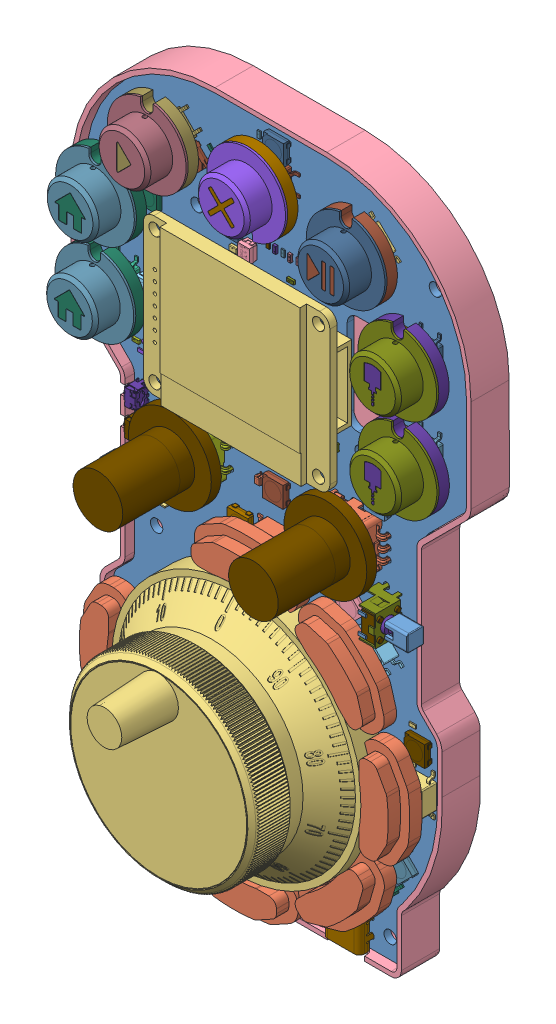
SolidWorks assembly jog3k, configuration Default. Lengths in mm.
Overall size (115.24 180.92 49.48).
240 component instances, 221 part files, 38 mates.
Components (placement in the parent):
- I2C_Jog_Controller-4: I2C_Jog_Controller [Default] at origin size (94.01 162 28.4)
  - Open CASCADE STEP translator 7.5 412-1: Open CASCADE STEP translator 7.5 412 [Default] at origin size (94.01 162 1.63)
  - Open CASCADE STEP translator 7.5 413-1: Open CASCADE STEP translator 7.5 413 [Default] at origin size (10 6 5.08)
  - Open CASCADE STEP translator 7.5 414-1: Open CASCADE STEP translator 7.5 414 [Default] at origin size (6 10 5.08)
  - Open CASCADE STEP translator 7.5 415-1: Open CASCADE STEP translator 7.5 415 [Default] at origin size (6 10 5.08)
  - Open CASCADE STEP translator 7.5 416-1: Open CASCADE STEP translator 7.5 416 [Default] at origin size (10 6 5.08)
  - Open CASCADE STEP translator 7.5 417-1: Open CASCADE STEP translator 7.5 417 [Default] at origin size (1.7 0.8 0.58)
  - Open CASCADE STEP translator 7.5 418-1: Open CASCADE STEP translator 7.5 418 [Default] at origin size (1.77 1.77 0.58)
  - Open CASCADE STEP translator 7.5 419-1: Open CASCADE STEP translator 7.5 419 [Default] at origin size (1.77 1.77 0.58)
  - Open CASCADE STEP translator 7.5 420-1: Open CASCADE STEP translator 7.5 420 [Default] at origin size (5 5.4 1.7)
  - Open CASCADE STEP translator 7.5 421-1: Open CASCADE STEP translator 7.5 421 [Default] at origin size (0.8 1.7 0.58)
  - Open CASCADE STEP translator 7.5 422-1: Open CASCADE STEP translator 7.5 422 [Default] at origin size (0.8 1.6 0.31)
  - Open CASCADE STEP translator 7.5 423-1: Open CASCADE STEP translator 7.5 423 [Default] at origin size (0.8 1.6 0.31)
  - Open CASCADE STEP translator 7.5 424-1: Open CASCADE STEP translator 7.5 424 [Default] at origin size (5 5.4 1.7)
  - Open CASCADE STEP translator 7.5 425-1: Open CASCADE STEP translator 7.5 425 [Default] at origin size (6 10 5.08)
  - Open CASCADE STEP translator 7.5 426-1: Open CASCADE STEP translator 7.5 426 [Default] at origin size (1.7 0.8 0.58)
  - Open CASCADE STEP translator 7.5 427-1: Open CASCADE STEP translator 7.5 427 [Default] at origin size (1.6 0.8 0.31)
  - Open CASCADE STEP translator 7.5 428-1: Open CASCADE STEP translator 7.5 428 [Default] at origin size (1.6 0.8 0.31)
  - Open CASCADE STEP translator 7.5 429-1: Open CASCADE STEP translator 7.5 429 [Default] at origin size (5.4 5 1.7)
  - Open CASCADE STEP translator 7.5 430-1: Open CASCADE STEP translator 7.5 430 [Default] at origin size (0.8 1.7 0.58)
  - Open CASCADE STEP translator 7.5 431-1: Open CASCADE STEP translator 7.5 431 [Default] at origin size (0.8 1.6 0.31)
  - Open CASCADE STEP translator 7.5 432-1: Open CASCADE STEP translator 7.5 432 [Default] at origin size (1.6 0.8 0.31)
  - Open CASCADE STEP translator 7.5 433-1: Open CASCADE STEP translator 7.5 433 [Default] at origin size (7.07 7.07 1.7)
  - Open CASCADE STEP translator 7.5 434-1: Open CASCADE STEP translator 7.5 434 [Default] at origin size (10.75 10.75 5.08)
  - Open CASCADE STEP translator 7.5 435-1: Open CASCADE STEP translator 7.5 435 [Default] at origin size (1.7 0.8 0.58)
  - Open CASCADE STEP translator 7.5 436-1: Open CASCADE STEP translator 7.5 436 [Default] at origin size (1.6 0.8 0.31)
  - Open CASCADE STEP translator 7.5 437-1: Open CASCADE STEP translator 7.5 437 [Default] at origin size (1.69 1.7 0.31)
  - Open CASCADE STEP translator 7.5 438-1: Open CASCADE STEP translator 7.5 438 [Default] at origin size (5 5.4 1.7)
  - Open CASCADE STEP translator 7.5 439-1: Open CASCADE STEP translator 7.5 439 [Default] at origin size (6 10 5.08)
  - Open CASCADE STEP translator 7.5 440-1: Open CASCADE STEP translator 7.5 440 [Default] at origin size (0.8 1.7 0.58)
  - Open CASCADE STEP translator 7.5 441-1: Open CASCADE STEP translator 7.5 441 [Default] at origin size (0.8 1.6 0.31)
  - Open CASCADE STEP translator 7.5 442-1: Open CASCADE STEP translator 7.5 442 [Default] at origin size (1.6 0.8 0.31)
  - Open CASCADE STEP translator 7.5 443-1: Open CASCADE STEP translator 7.5 443 [Default] at origin size (7.07 7.07 1.7)
  - Open CASCADE STEP translator 7.5 444-1: Open CASCADE STEP translator 7.5 444 [Default] at origin size (10.75 10.75 5.08)
  - Open CASCADE STEP translator 7.5 445-1: Open CASCADE STEP translator 7.5 445 [Default] at origin size (0.8 1.7 0.58)
  - Open CASCADE STEP translator 7.5 446-1: Open CASCADE STEP translator 7.5 446 [Default] at origin size (0.8 1.6 0.31)
  - Open CASCADE STEP translator 7.5 447-1: Open CASCADE STEP translator 7.5 447 [Default] at origin size (1.69 1.69 0.31)
  - Open CASCADE STEP translator 7.5 448-1: Open CASCADE STEP translator 7.5 448 [Default] at origin size (5.4 5 1.7)
  - Open CASCADE STEP translator 7.5 449-1: Open CASCADE STEP translator 7.5 449 [Default] at origin size (0.8 1.7 0.58)
  - Open CASCADE STEP translator 7.5 450-1: Open CASCADE STEP translator 7.5 450 [Default] at origin size (0.8 1.6 0.31)
  - Open CASCADE STEP translator 7.5 451-1: Open CASCADE STEP translator 7.5 451 [Default] at origin size (1.6 0.8 0.31)
  - Open CASCADE STEP translator 7.5 452-1: Open CASCADE STEP translator 7.5 452 [Default] at origin size (5 5.4 1.7)
  - Open CASCADE STEP translator 7.5 453-1: Open CASCADE STEP translator 7.5 453 [Default] at origin size (6 10 5.08)
  - Open CASCADE STEP translator 7.5 454-1: Open CASCADE STEP translator 7.5 454 [Default] at origin size (0.8 1.7 0.58)
  - Open CASCADE STEP translator 7.5 455-1: Open CASCADE STEP translator 7.5 455 [Default] at origin size (0.8 1.6 0.31)
  - Open CASCADE STEP translator 7.5 456-1: Open CASCADE STEP translator 7.5 456 [Default] at origin size (1.6 0.8 0.31)
  - Open CASCADE STEP translator 7.5 457-1: Open CASCADE STEP translator 7.5 457 [Default] at origin size (5.4 5 1.7)
  - Open CASCADE STEP translator 7.5 458-1: Open CASCADE STEP translator 7.5 458 [Default] at origin size (10 6 5.08)
  - Open CASCADE STEP translator 7.5 459-1: Open CASCADE STEP translator 7.5 459 [Default] at origin size (0.8 1.7 0.58)
  - Open CASCADE STEP translator 7.5 460-1: Open CASCADE STEP translator 7.5 460 [Default] at origin size (0.8 1.6 0.31)
  - Open CASCADE STEP translator 7.5 461-1: Open CASCADE STEP translator 7.5 461 [Default] at origin size (0.8 1.6 0.31)
  - Open CASCADE STEP translator 7.5 462-1: Open CASCADE STEP translator 7.5 462 [Default] at origin size (5 5.4 1.7)
  - Open CASCADE STEP translator 7.5 463-1: Open CASCADE STEP translator 7.5 463 [Default] at origin size (6 10 5.08)
  - Open CASCADE STEP translator 7.5 464-1: Open CASCADE STEP translator 7.5 464 [Default] at origin size (0.8 1.7 0.58)
  - Open CASCADE STEP translator 7.5 465-1: Open CASCADE STEP translator 7.5 465 [Default] at origin size (0.8 1.6 0.31)
  - Open CASCADE STEP translator 7.5 466-1: Open CASCADE STEP translator 7.5 466 [Default] at origin size (1.6 0.8 0.31)
  - Open CASCADE STEP translator 7.5 467-1: Open CASCADE STEP translator 7.5 467 [Default] at origin size (7.07 7.07 1.7)
  - Open CASCADE STEP translator 7.5 468-1: Open CASCADE STEP translator 7.5 468 [Default] at origin size (10.75 10.75 5.08)
  - Open CASCADE STEP translator 7.5 469-1: Open CASCADE STEP translator 7.5 469 [Default] at origin size (0.8 1.7 0.58)
  - Open CASCADE STEP translator 7.5 470-1: Open CASCADE STEP translator 7.5 470 [Default] at origin size (0.8 1.6 0.31)
  - Open CASCADE STEP translator 7.5 471-1: Open CASCADE STEP translator 7.5 471 [Default] at origin size (1.7 1.69 0.31)
  - Open CASCADE STEP translator 7.5 472-1: Open CASCADE STEP translator 7.5 472 [Default] at origin size (5 5.4 1.7)
  - Open CASCADE STEP translator 7.5 473-1: Open CASCADE STEP translator 7.5 473 [Default] at origin size (0.8 1.7 0.58)
  - Open CASCADE STEP translator 7.5 474-1: Open CASCADE STEP translator 7.5 474 [Default] at origin size (0.8 1.6 0.31)
  - Open CASCADE STEP translator 7.5 475-1: Open CASCADE STEP translator 7.5 475 [Default] at origin size (1.6 0.8 0.31)
  - Open CASCADE STEP translator 7.5 476-1: Open CASCADE STEP translator 7.5 476 [Default] at origin size (7.07 7.07 1.7)
  - Open CASCADE STEP translator 7.5 477-1: Open CASCADE STEP translator 7.5 477 [Default] at origin size (10.75 10.75 5.08)
  - Open CASCADE STEP translator 7.5 478-1: Open CASCADE STEP translator 7.5 478 [Default] at origin size (0.8 1.7 0.58)
  - Open CASCADE STEP translator 7.5 479-1: Open CASCADE STEP translator 7.5 479 [Default] at origin size (0.8 1.6 0.31)
  - Open CASCADE STEP translator 7.5 480-1: Open CASCADE STEP translator 7.5 480 [Default] at origin size (1.7 1.69 0.31)
  - Open CASCADE STEP translator 7.5 481-1: Open CASCADE STEP translator 7.5 481 [Default] at origin size (6.25 8.7 11.7)
  - Open CASCADE STEP translator 7.5 482-1: Open CASCADE STEP translator 7.5 482 [Default] at origin size (4 3.5 3.5)
  - Open CASCADE STEP translator 7.5 483-1: Open CASCADE STEP translator 7.5 483 [Default] at origin size (3.91 6.01 6.01)
  - Open CASCADE STEP translator 7.5 484-1: Open CASCADE STEP translator 7.5 484 [Default] at origin size (1.9 5.2 11.6)
  - Open CASCADE STEP translator 7.5 485-1: Open CASCADE STEP translator 7.5 485 [Default] at origin size (3 0.02 4.74)
  - Open CASCADE STEP translator 7.5 486-1: Open CASCADE STEP translator 7.5 486 [Default] at origin size (6.25 8.7 11.7)
  - Open CASCADE STEP translator 7.5 487-1: Open CASCADE STEP translator 7.5 487 [Default] at origin size (4 3.5 3.5)
  - Open CASCADE STEP translator 7.5 488-1: Open CASCADE STEP translator 7.5 488 [Default] at origin size (3.91 6.01 6.01)
  - Open CASCADE STEP translator 7.5 489-1: Open CASCADE STEP translator 7.5 489 [Default] at origin size (1.9 5.2 11.6)
  - Open CASCADE STEP translator 7.5 490-1: Open CASCADE STEP translator 7.5 490 [Default] at origin size (3 0.02 4.74)
  - Open CASCADE STEP translator 7.5 491-1: Open CASCADE STEP translator 7.5 491 [Default] at origin size (7.31 7.31 2.01)
  - Open CASCADE STEP translator 7.5 492-1: Open CASCADE STEP translator 7.5 492 [Default] at origin size (1.77 1.77 0.58)
  - Open CASCADE STEP translator 7.5 493-1: Open CASCADE STEP translator 7.5 493 [Default] at origin size (1.77 1.77 0.58)
  - Open CASCADE STEP translator 7.5 494-1: Open CASCADE STEP translator 7.5 494 [Default] at origin size (1.69 1.69 0.31)
  - Open CASCADE STEP translator 7.5 495-1: Open CASCADE STEP translator 7.5 495 [Default] at origin size (1.69 1.7 0.31)
  - Open CASCADE STEP translator 7.5 496-1: Open CASCADE STEP translator 7.5 496 [Default] at origin size (1.7 1.69 0.31)
  - Open CASCADE STEP translator 7.5 497-1: Open CASCADE STEP translator 7.5 497 [Default] at origin size (1.7 0.8 0.58)
  - Open CASCADE STEP translator 7.5 498-1: Open CASCADE STEP translator 7.5 498 [Default] at origin size (1.6 0.8 0.31)
  - Open CASCADE STEP translator 7.5 499-1: Open CASCADE STEP translator 7.5 499 [Default] at origin size (1.7 0.8 0.58)
  - Open CASCADE STEP translator 7.5 500-1: Open CASCADE STEP translator 7.5 500 [Default] at origin size (0.8 1.7 0.58)
  - Open CASCADE STEP translator 7.5 501-1: Open CASCADE STEP translator 7.5 501 [Default] at origin size (0.8 1.7 0.58)
  - Open CASCADE STEP translator 7.5 502-1: Open CASCADE STEP translator 7.5 502 [Default] at origin size (1.7 0.8 0.58)
  - Open CASCADE STEP translator 7.5 503-1: Open CASCADE STEP translator 7.5 503 [Default] at origin size (1.7 0.8 0.58)
  - Open CASCADE STEP translator 7.5 504-1: Open CASCADE STEP translator 7.5 504 [Default] at origin size (1.7 0.8 0.58)
  - Open CASCADE STEP translator 7.5 505-1: Open CASCADE STEP translator 7.5 505 [Default] at origin size (0.8 1.6 0.31)
  - Open CASCADE STEP translator 7.5 506-1: Open CASCADE STEP translator 7.5 506 [Default] at origin size (1.6 0.8 0.31)
  - Open CASCADE STEP translator 7.5 507-1: Open CASCADE STEP translator 7.5 507 [Default] at origin size (1.6 0.8 0.31)
  - Open CASCADE STEP translator 7.5 508-1: Open CASCADE STEP translator 7.5 508 [Default] at origin size (1.6 0.8 0.31)
  - Open CASCADE STEP translator 7.5 509-1: Open CASCADE STEP translator 7.5 509 [Default] at origin size (1.6 0.8 0.31)
  - Open CASCADE STEP translator 7.5 510-1: Open CASCADE STEP translator 7.5 510 [Default] at origin size (1.6 0.8 0.31)
  - Open CASCADE STEP translator 7.5 511-1: Open CASCADE STEP translator 7.5 511 [Default] at origin size (3.1 1.8 1.25)
  - Open CASCADE STEP translator 7.5 512-1: Open CASCADE STEP translator 7.5 512 [Default] at origin size (5.4 5 1.7)
  - Open CASCADE STEP translator 7.5 513-1: Open CASCADE STEP translator 7.5 513 [Default] at origin size (0.8 1.7 0.58)
  - Open CASCADE STEP translator 7.5 514-1: Open CASCADE STEP translator 7.5 514 [Default] at origin size (0.8 1.7 0.58)
  - Open CASCADE STEP translator 7.5 515-1: Open CASCADE STEP translator 7.5 515 [Default] at origin size (1.77 1.77 0.58)
  - Open CASCADE STEP translator 7.5 516-1: Open CASCADE STEP translator 7.5 516 [Default] at origin size (1.77 1.77 0.58)
  - Open CASCADE STEP translator 7.5 517-1: Open CASCADE STEP translator 7.5 517 [Default] at origin size (1.7 0.8 0.58)
  - Open CASCADE STEP translator 7.5 518-1: Open CASCADE STEP translator 7.5 518 [Default] at origin size (1.77 1.77 0.58)
  - Open CASCADE STEP translator 7.5 519-1: Open CASCADE STEP translator 7.5 519 [Default] at origin size (1.77 1.77 0.58)
  - Open CASCADE STEP translator 7.5 520-1: Open CASCADE STEP translator 7.5 520 [Default] at origin size (1.77 1.77 0.58)
  - Open CASCADE STEP translator 7.5 521-1: Open CASCADE STEP translator 7.5 521 [Default] at origin size (1.25 2.74 1.12)
  - Open CASCADE STEP translator 7.5 522-1: Open CASCADE STEP translator 7.5 522 [Default] at origin size (2 1.25 0.8)
  - Open CASCADE STEP translator 7.5 523-1: Open CASCADE STEP translator 7.5 523 [Default] at origin size (2.93 3.7 2.03)
  - Open CASCADE STEP translator 7.5 524-1: Open CASCADE STEP translator 7.5 524 [Default] at origin size (1.25 2 0.8)
  - Open CASCADE STEP translator 7.5 525-1: Open CASCADE STEP translator 7.5 525 [Default] at origin size (1.69 1.7 0.31)
  - Open CASCADE STEP translator 7.5 526-1: Open CASCADE STEP translator 7.5 526 [Default] at origin size (1.69 1.69 0.31)
  - Open CASCADE STEP translator 7.5 527-1: Open CASCADE STEP translator 7.5 527 [Default] at origin size (1.7 1.69 0.31)
  - Open CASCADE STEP translator 7.5 528-1: Open CASCADE STEP translator 7.5 528 [Default] at origin size (1.7 1.69 0.31)
  - Open CASCADE STEP translator 7.5 529-1: Open CASCADE STEP translator 7.5 529 [Default] at origin size (1.69 1.69 0.31)
  - Open CASCADE STEP translator 7.5 530-1: Open CASCADE STEP translator 7.5 530 [Default] at origin size (1.7 1.7 0.31)
  - Open CASCADE STEP translator 7.5 531-1: Open CASCADE STEP translator 7.5 531 [Default] at origin size (1.7 1.69 0.31)
  - Open CASCADE STEP translator 7.5 532-1: Open CASCADE STEP translator 7.5 532 [Default] at origin size (1.7 1.69 0.31)
  - Open CASCADE STEP translator 7.5 533-1: Open CASCADE STEP translator 7.5 533 [Default] at origin size (1.7 1.69 0.31)
  - Open CASCADE STEP translator 7.5 534-1: Open CASCADE STEP translator 7.5 534 [Default] at origin size (1.69 1.69 0.31)
  - Open CASCADE STEP translator 7.5 535-1: Open CASCADE STEP translator 7.5 535 [Default] at origin size (1.7 1.7 0.31)
  - Open CASCADE STEP translator 7.5 536-1: Open CASCADE STEP translator 7.5 536 [Default] at origin size (0.8 1.6 0.31)
  - Open CASCADE STEP translator 7.5 537-1: Open CASCADE STEP translator 7.5 537 [Default] at origin size (0.8 1.6 0.31)
  - Open CASCADE STEP translator 7.5 538-1: Open CASCADE STEP translator 7.5 538 [Default] at origin size (2.3 2.24 0.84)
  - Open CASCADE STEP translator 7.5 539-1: Open CASCADE STEP translator 7.5 539 [Default] at origin size (0.8 1.6 0.31)
  - Open CASCADE STEP translator 7.5 540-1: Open CASCADE STEP translator 7.5 540 [Default] at origin size (0.6 1 0.21)
  - Open CASCADE STEP translator 7.5 541-1: Open CASCADE STEP translator 7.5 541 [Default] at origin size (0.8 1.6 0.31)
  - Open CASCADE STEP translator 7.5 542-1: Open CASCADE STEP translator 7.5 542 [Default] at origin size (1.77 1.77 0.58)
  - Open CASCADE STEP translator 7.5 543-1: Open CASCADE STEP translator 7.5 543 [Default] at origin size (0.8 1.6 0.31)
  - Open CASCADE STEP translator 7.5 544-1: Open CASCADE STEP translator 7.5 544 [Default] at origin size (1.7 0.8 0.58)
  - Open CASCADE STEP translator 7.5 545-1: Open CASCADE STEP translator 7.5 545 [Default] at origin size (1.6 0.8 0.31)
  - Open CASCADE STEP translator 7.5 546-1: Open CASCADE STEP translator 7.5 546 [Default] at origin size (8.94 7.91 4.3)
  - Open CASCADE STEP translator 7.5 547-1: Open CASCADE STEP translator 7.5 547 [Default] at origin size (3.2 2.5 0.8)
  - Open CASCADE STEP translator 7.5 548-1: Open CASCADE STEP translator 7.5 548 [Default] at origin size (3.36 2.66 0.1)
  - Open CASCADE STEP translator 7.5 549-1: Open CASCADE STEP translator 7.5 549 [Default] at origin size (0.88 0.88 0)
  - Open CASCADE STEP translator 7.5 550-1: Open CASCADE STEP translator 7.5 550 [Default] at origin size (9.9 9.9 0.9)
  - Open CASCADE STEP translator 7.5 551-1: Open CASCADE STEP translator 7.5 551 [Default] at origin size (4.28 4.53 0)
  - Open CASCADE STEP translator 7.5 552-1: Open CASCADE STEP translator 7.5 552 [Default] at origin size (0.42 0.42 0.2)
  - Open CASCADE STEP translator 7.5 553-1: Open CASCADE STEP translator 7.5 553 [Default] at origin size (0.42 0.42 0.2)
  - Open CASCADE STEP translator 7.5 554-1: Open CASCADE STEP translator 7.5 554 [Default] at origin size (0.42 0.42 0.2)
  - Open CASCADE STEP translator 7.5 555-1: Open CASCADE STEP translator 7.5 555 [Default] at origin size (0.42 0.42 0.2)
  - Open CASCADE STEP translator 7.5 556-1: Open CASCADE STEP translator 7.5 556 [Default] at origin size (0.42 0.42 0.2)
  - Open CASCADE STEP translator 7.5 557-1: Open CASCADE STEP translator 7.5 557 [Default] at origin size (0.42 0.42 0.2)
  - Open CASCADE STEP translator 7.5 558-1: Open CASCADE STEP translator 7.5 558 [Default] at origin size (0.42 0.42 0.2)
  - Open CASCADE STEP translator 7.5 559-1: Open CASCADE STEP translator 7.5 559 [Default] at origin size (0.42 0.42 0.2)
  - Open CASCADE STEP translator 7.5 560-1: Open CASCADE STEP translator 7.5 560 [Default] at origin size (0.42 0.42 0.2)
  - Open CASCADE STEP translator 7.5 561-1: Open CASCADE STEP translator 7.5 561 [Default] at origin size (0.42 0.42 0.2)
  - Open CASCADE STEP translator 7.5 562-1: Open CASCADE STEP translator 7.5 562 [Default] at origin size (0.42 0.42 0.2)
  - Open CASCADE STEP translator 7.5 563-1: Open CASCADE STEP translator 7.5 563 [Default] at origin size (0.42 0.42 0.2)
  - Open CASCADE STEP translator 7.5 564-1: Open CASCADE STEP translator 7.5 564 [Default] at origin size (0.42 0.42 0.2)
  - Open CASCADE STEP translator 7.5 565-1: Open CASCADE STEP translator 7.5 565 [Default] at origin size (0.42 0.42 0.2)
  - Open CASCADE STEP translator 7.5 566-1: Open CASCADE STEP translator 7.5 566 [Default] at origin size (0.42 0.42 0.2)
  - Open CASCADE STEP translator 7.5 567-1: Open CASCADE STEP translator 7.5 567 [Default] at origin size (0.42 0.42 0.2)
  - Open CASCADE STEP translator 7.5 568-1: Open CASCADE STEP translator 7.5 568 [Default] at origin size (0.42 0.42 0.2)
  - Open CASCADE STEP translator 7.5 569-1: Open CASCADE STEP translator 7.5 569 [Default] at origin size (0.42 0.42 0.2)
  - Open CASCADE STEP translator 7.5 570-1: Open CASCADE STEP translator 7.5 570 [Default] at origin size (0.42 0.42 0.2)
  - Open CASCADE STEP translator 7.5 571-1: Open CASCADE STEP translator 7.5 571 [Default] at origin size (0.42 0.42 0.2)
  - Open CASCADE STEP translator 7.5 572-1: Open CASCADE STEP translator 7.5 572 [Default] at origin size (0.42 0.42 0.2)
  - Open CASCADE STEP translator 7.5 573-1: Open CASCADE STEP translator 7.5 573 [Default] at origin size (0.42 0.42 0.2)
  - Open CASCADE STEP translator 7.5 574-1: Open CASCADE STEP translator 7.5 574 [Default] at origin size (0.42 0.42 0.2)
  - Open CASCADE STEP translator 7.5 575-1: Open CASCADE STEP translator 7.5 575 [Default] at origin size (0.42 0.42 0.2)
  - Open CASCADE STEP translator 7.5 576-1: Open CASCADE STEP translator 7.5 576 [Default] at origin size (0.42 0.42 0.2)
  - Open CASCADE STEP translator 7.5 577-1: Open CASCADE STEP translator 7.5 577 [Default] at origin size (0.42 0.42 0.2)
  - Open CASCADE STEP translator 7.5 578-1: Open CASCADE STEP translator 7.5 578 [Default] at origin size (0.42 0.42 0.2)
  - Open CASCADE STEP translator 7.5 579-1: Open CASCADE STEP translator 7.5 579 [Default] at origin size (0.42 0.42 0.2)
  - Open CASCADE STEP translator 7.5 580-1: Open CASCADE STEP translator 7.5 580 [Default] at origin size (0.42 0.42 0.2)
  - Open CASCADE STEP translator 7.5 581-1: Open CASCADE STEP translator 7.5 581 [Default] at origin size (0.42 0.42 0.2)
  - Open CASCADE STEP translator 7.5 582-1: Open CASCADE STEP translator 7.5 582 [Default] at origin size (0.42 0.42 0.2)
  - Open CASCADE STEP translator 7.5 583-1: Open CASCADE STEP translator 7.5 583 [Default] at origin size (0.42 0.42 0.2)
  - Open CASCADE STEP translator 7.5 584-1: Open CASCADE STEP translator 7.5 584 [Default] at origin size (0.42 0.42 0.2)
  - Open CASCADE STEP translator 7.5 585-1: Open CASCADE STEP translator 7.5 585 [Default] at origin size (0.42 0.42 0.2)
  - Open CASCADE STEP translator 7.5 586-1: Open CASCADE STEP translator 7.5 586 [Default] at origin size (0.42 0.42 0.2)
  - Open CASCADE STEP translator 7.5 587-1: Open CASCADE STEP translator 7.5 587 [Default] at origin size (0.42 0.42 0.2)
  - Open CASCADE STEP translator 7.5 588-1: Open CASCADE STEP translator 7.5 588 [Default] at origin size (0.42 0.42 0.2)
  - Open CASCADE STEP translator 7.5 589-1: Open CASCADE STEP translator 7.5 589 [Default] at origin size (0.42 0.42 0.2)
  - Open CASCADE STEP translator 7.5 590-1: Open CASCADE STEP translator 7.5 590 [Default] at origin size (0.42 0.42 0.2)
  - Open CASCADE STEP translator 7.5 591-1: Open CASCADE STEP translator 7.5 591 [Default] at origin size (0.42 0.42 0.2)
  - Open CASCADE STEP translator 7.5 592-1: Open CASCADE STEP translator 7.5 592 [Default] at origin size (0.42 0.42 0.2)
  - Open CASCADE STEP translator 7.5 593-1: Open CASCADE STEP translator 7.5 593 [Default] at origin size (0.42 0.42 0.2)
  - Open CASCADE STEP translator 7.5 594-1: Open CASCADE STEP translator 7.5 594 [Default] at origin size (0.42 0.42 0.2)
  - Open CASCADE STEP translator 7.5 595-1: Open CASCADE STEP translator 7.5 595 [Default] at origin size (0.42 0.42 0.2)
  - Open CASCADE STEP translator 7.5 596-1: Open CASCADE STEP translator 7.5 596 [Default] at origin size (0.42 0.42 0.2)
  - Open CASCADE STEP translator 7.5 597-1: Open CASCADE STEP translator 7.5 597 [Default] at origin size (0.42 0.42 0.2)
  - Open CASCADE STEP translator 7.5 598-1: Open CASCADE STEP translator 7.5 598 [Default] at origin size (0.42 0.42 0.2)
  - Open CASCADE STEP translator 7.5 599-1: Open CASCADE STEP translator 7.5 599 [Default] at origin size (0.42 0.42 0.2)
  - Open CASCADE STEP translator 7.5 600-1: Open CASCADE STEP translator 7.5 600 [Default] at origin size (0.42 0.42 0.2)
  - Open CASCADE STEP translator 7.5 601-1: Open CASCADE STEP translator 7.5 601 [Default] at origin size (0.42 0.42 0.2)
  - Open CASCADE STEP translator 7.5 602-1: Open CASCADE STEP translator 7.5 602 [Default] at origin size (0.42 0.42 0.2)
  - Open CASCADE STEP translator 7.5 603-1: Open CASCADE STEP translator 7.5 603 [Default] at origin size (0.42 0.42 0.2)
  - Open CASCADE STEP translator 7.5 604-1: Open CASCADE STEP translator 7.5 604 [Default] at origin size (0.42 0.42 0.2)
  - Open CASCADE STEP translator 7.5 605-1: Open CASCADE STEP translator 7.5 605 [Default] at origin size (0.42 0.42 0.2)
  - Open CASCADE STEP translator 7.5 606-1: Open CASCADE STEP translator 7.5 606 [Default] at origin size (0.42 0.42 0.2)
  - Open CASCADE STEP translator 7.5 607-1: Open CASCADE STEP translator 7.5 607 [Default] at origin size (0.42 0.42 0.2)
  - Open CASCADE STEP translator 7.5 608-1: Open CASCADE STEP translator 7.5 608 [Default] at origin size (3.55 4.5 3.8)
  - Open CASCADE STEP translator 7.5 609-1: Open CASCADE STEP translator 7.5 609 [Default] at origin size (3.55 4.5 3.8)
  - Open CASCADE STEP translator 7.5 610-1: Open CASCADE STEP translator 7.5 610 [Default] at origin size (5.4 5 1.7)
  - Open CASCADE STEP translator 7.5 611-1: Open CASCADE STEP translator 7.5 611 [Default] at origin size (14.98 13.1 28.2)
  - Open CASCADE STEP translator 7.5 612-1: Open CASCADE STEP translator 7.5 612 [Default] at origin size (45 37.5 9.4)
  - Open CASCADE STEP translator 7.5 613-1: Open CASCADE STEP translator 7.5 613 [Default] at origin size (5.23 5.23 1.8)
  - Open CASCADE STEP translator 7.5 614-1: Open CASCADE STEP translator 7.5 614 [Default] at origin size (7.8 4.23 1.11)
  - Open CASCADE STEP translator 7.5 616-1: Open CASCADE STEP translator 7.5 616 [Default] at origin size (5.4 5 1.7)
  - Open CASCADE STEP translator 7.5 617-1: Open CASCADE STEP translator 7.5 617 [Default] at origin size (14.98 13.1 28.2)
- halt_button-1: halt_button [Default] at (7.9129 120.3247 -3.7629) x (-1 0 0) z (0 0 1) size (19 18.88 9)
  - Halt Button Cover-1: Halt Button Cover [Default] at (7.9127 9.3246 8.8429) size (19 18.88 6.5)
  - Halt Button Lightpipe-1: Halt Button Lightpipe [Default] at (7.9127 9.3246 8.8429) size (19 18.88 9)
- Hold_button-1: Hold_button [Default] at (18.335 99.1832 -4.6146) size (19 18.88 9)
  - Hold Button Cover-2: Hold Button Cover [Default] at (5.6648 9.8169 9.6946) size (19 18.88 6.5)
  - Hold Button Lightpipe-1: Hold Button Lightpipe [Default] at (5.6648 9.8169 9.6946) size (19 18.88 9)
- start_button-1: start_button [Default] at (-32.4958 98.8123 -8.5785) size (19 18.88 9)
  - Start Button Lightpipe-1: Start Button Lightpipe [Default] at (8.4957 10.1876 13.6585) size (19 18.88 9)
  - Start Button Cover-1: Start Button Cover [Default] at (8.4957 10.1876 13.6585) size (19 18.88 6.5)
- Home_button-1: Home_button [Default] at (-43.1593 60.9431 -3.5645) size (19 18.88 9)
  - Home Button Cover-1: Home Button Cover [Default] at (6.5093 10.7068 8.6445) size (19 18.88 6.5)
  - Home Button Lightpipe-1: Home Button Lightpipe [Default] at (6.5093 10.7068 8.6445) size (19 18.88 9)
- spindle_button-1: spindle_button [Default] at (35.5679 62.8775 -7.999) size (19 18.88 9)
  - Spindle Button Cover-1: Spindle Button Cover [Default] at (0.982 8.4726 13.079) size (19 18.88 6.5)
  - Spindle Button Lightpipe-1: Spindle Button Lightpipe [Default] at (0.982 8.4726 13.079) size (19 18.88 9)
- spindle_button-2: spindle_button [Default] at (35.5179 83.5275 -7.999) size (19 18.88 9)
  - Spindle Button Cover-1: Spindle Button Cover [Default] at (0.982 8.4726 13.079) size (19 18.88 6.5)
  - Spindle Button Lightpipe-1: Spindle Button Lightpipe [Default] at (0.982 8.4726 13.079) size (19 18.88 9)
- Home_button-2: Home_button [Default] at (-43.0093 81.2931 -3.5645) size (19 18.88 9)
  - Home Button Cover-1: Home Button Cover [Default] at (6.5093 10.7068 8.6445) size (19 18.88 6.5)
  - Home Button Lightpipe-1: Home Button Lightpipe [Default] at (6.5093 10.7068 8.6445) size (19 18.88 9)
- simple_rotary_knob^jog3k-1: simple_rotary_knob^jog3k [Default] at (0 0 4.3036) x (1 0 0) z (0 0 1) size (20 20 19.8)
- b32-1010-1: b32-1010 [Default] at (31.675 34.35 4.35) x (0 -1 0) z (0 0 1) size (4 5.5 4)
- b32-1010-2: b32-1010 [Default] at (-31.675 34.35 4.35) x (0 -1 0) z (0 0 -1) size (4 5.5 4)
- simple_rotary_knob^jog3k-2: simple_rotary_knob^jog3k [Default] at (0 92 4.3036) x (-1 0 0) z (0 0 1) size (20 20 19.8)
- simple_direction_button^jog3k-1: simple_direction_button^jog3k [Default] at (0 0 5.08) size (25 57.62 6)
- simple_direction_button^jog3k-2: simple_direction_button^jog3k [Default] at (0 0.0057 5.08) x (0 1 0) z (0 0 1) size (25 57.62 6)
- simple_direction_button^jog3k-3: simple_direction_button^jog3k [Default] at (-0.0005 -0.1857 5.08) x (0 -1 0) z (0 0 1) size (25 57.62 6)
- simple_direction_button^jog3k-4: simple_direction_button^jog3k [Default] at (-0.0084 0 5.08) x (-1 0 0) z (0 0 1) size (25 57.62 6)
- simple_direction_button^jog3k-5: simple_direction_button^jog3k [Default] at (-0.0164 -0.0171 5.08) x (0.707107 -0.707107 0) z (0 0 1) size (25 57.62 6)
- simple_direction_button^jog3k-6: simple_direction_button^jog3k [Default] at (-0.0004 -0.0005 5.08) x (-0.707107 -0.707107 0) z (0 0 1) size (25 57.62 6)
- cast_top^jog3k-1: cast_top^jog3k [Default] at (0 0 8.08) size (96.61 164.6 10.08) (hidden)
- Rotary Pulse Encoder 60mm-1: Rotary Pulse Encoder 60mm [Default] at (0.1444 0.0143 4.5) x (0.999984 0.005717 0) z (0.005717 -0.999984 0) size (60.35 49.1 60.35)
- cast_bottom^jog3k-1: cast_bottom^jog3k [Default] at (0 0 -5.6264) x (-1 0 0) z (0 0 -1) size (96.61 164.6 9.23)
Mates (geometry in assembly coordinates):
- Coincident1: coincident anti-aligned: plane of I2C_Jog_Controller-4/Open CASCADE STEP translator 7.5 458-1 through (0.0001 111 5.08) normal (0 0 1); plane of halt_button-1/Halt Button Lightpipe-1 through (0.0001 111 5.08) normal (0 0 -1)
- Concentric1: concentric anti-aligned: cylinder of I2C_Jog_Controller-4/Open CASCADE STEP translator 7.5 458-1 through (0.0001 111 3.61) axis (0 0 1) radius 1.75; cylinder of halt_button-1/Halt Button Lightpipe-1 through (0.0001 111 7.58) axis (0 0 -1) radius 9.5
- Coincident2: coincident anti-aligned: plane of I2C_Jog_Controller-4/Open CASCADE STEP translator 7.5 477-1 through (-24.0001 108.9999 5.08) normal (0 0 1); plane of start_button-1/Start Button Lightpipe-1 through (-24.0001 108.9999 5.08) normal (0 0 -1)
- Concentric2: concentric anti-aligned: cylinder of I2C_Jog_Controller-4/Open CASCADE STEP translator 7.5 477-1 through (-24.0001 108.9999 3.61) axis (0 0 1) radius 1.75; cylinder of start_button-1/Start Button Lightpipe-1 through (-24.0001 108.9999 7.58) axis (0 0 -1) radius 9.5
- Coincident3: coincident anti-aligned: plane of I2C_Jog_Controller-4/Open CASCADE STEP translator 7.5 468-1 through (23.9999 109.0001 5.08) normal (0 0 1); plane of Hold_button-1/Hold Button Lightpipe-1 through (23.9999 109.0001 5.08) normal (0 0 -1)
- Concentric3: concentric anti-aligned: cylinder of I2C_Jog_Controller-4/Open CASCADE STEP translator 7.5 468-1 through (23.9999 109.0001 3.61) axis (0 0 1) radius 1.75; cylinder of Hold_button-1/Hold Button Cover-2 through (23.9999 109.0001 14.08) axis (0 0 -1) radius 6.25
- Coincident4: coincident anti-aligned: plane of I2C_Jog_Controller-4/Open CASCADE STEP translator 7.5 425-1 through (36.55 71.3501 5.08) normal (0 0 1); plane of spindle_button-1/Spindle Button Lightpipe-1 through (36.55 71.3501 5.08) normal (0 0 -1)
- Concentric4: concentric anti-aligned: cylinder of I2C_Jog_Controller-4/Open CASCADE STEP translator 7.5 425-1 through (36.55 71.3501 3.61) axis (0 0 1) radius 1.75; cylinder of spindle_button-1/Spindle Button Lightpipe-1 through (36.55 71.3501 7.58) axis (0 0 -1) radius 9.5
- Coincident5: coincident anti-aligned: plane of I2C_Jog_Controller-4/Open CASCADE STEP translator 7.5 453-1 through (-36.65 71.6499 5.08) normal (0 0 1); plane of Home_button-1/Home Button Lightpipe-1 through (-36.65 71.6499 5.08) normal (0 0 -1)
- Concentric5: concentric anti-aligned: cylinder of I2C_Jog_Controller-4/Open CASCADE STEP translator 7.5 453-1 through (-36.65 71.6499 3.61) axis (0 0 1) radius 1.75; cylinder of Home_button-1/Home Button Cover-1 through (-36.65 71.6499 14.08) axis (0 0 -1) radius 6.25
- Coincident6: coincident anti-aligned: plane of I2C_Jog_Controller-4/Open CASCADE STEP translator 7.5 463-1 through (-36.5 91.9999 5.08) normal (0 0 1); plane of Home_button-2/Home Button Lightpipe-1 through (-36.5 91.9999 5.08) normal (0 0 -1)
- Concentric6: concentric anti-aligned: cylinder of I2C_Jog_Controller-4/Open CASCADE STEP translator 7.5 463-1 through (-36.5 91.9999 3.61) axis (0 0 1) radius 1.75; cylinder of Home_button-2/Home Button Lightpipe-1 through (-36.5 91.9999 7.58) axis (0 0 -1) radius 9.5
- Coincident7: coincident anti-aligned: plane of I2C_Jog_Controller-4/Open CASCADE STEP translator 7.5 439-1 through (36.5 92.0001 5.08) normal (0 0 1); plane of spindle_button-2/Spindle Button Lightpipe-1 through (36.5 92.0001 5.08) normal (0 0 -1)
- Concentric7: concentric anti-aligned: cylinder of I2C_Jog_Controller-4/Open CASCADE STEP translator 7.5 439-1 through (36.5 92.0001 3.61) axis (0 0 1) radius 1.75; cylinder of spindle_button-2/Spindle Button Cover-1 through (36.5 92.0001 14.08) axis (0 0 -1) radius 6.25
- Concentric8: concentric aligned: cylinder of I2C_Jog_Controller-4/Open CASCADE STEP translator 7.5 611-1 through (18.768 46 11.3036) axis (0 0 -1) radius 3.5; cylinder of simple_rotary_knob^jog3k-2 through (18.768 46 31.9742) axis (0 0 -1) radius 6
- Coincident12: coincident anti-aligned: plane of I2C_Jog_Controller-4/Open CASCADE STEP translator 7.5 482-1 through (34.475 35.5 5.6) normal (1 0 0); plane of b32-1010-1 through (34.475 34.35 4.35) normal (-1 0 0)
- Coincident15: coincident anti-aligned: plane of I2C_Jog_Controller-4/Open CASCADE STEP translator 7.5 482-1 through (32.675 33.1 5.6) normal (0 -1 0); plane of b32-1010-1 through (32.575 33.1 4.35) normal (0 1 0)
- Coincident17: coincident anti-aligned: plane of I2C_Jog_Controller-4/Open CASCADE STEP translator 7.5 482-1 through (32.675 33.1 5.6) normal (0 0 1); plane of b32-1010-1 through (32.575 34.35 5.6) normal (0 0 -1)
- Coincident18: coincident anti-aligned: plane of I2C_Jog_Controller-4/Open CASCADE STEP translator 7.5 487-1 through (-34.475 33.1 5.6) normal (-1 0 0); plane of b32-1010-2 through (-34.475 34.35 4.35) normal (1 0 0)
- Coincident19: coincident anti-aligned: plane of I2C_Jog_Controller-4/Open CASCADE STEP translator 7.5 487-1 through (-32.675 33.1 5.6) normal (0 -1 0); plane of b32-1010-2 through (-32.575 33.1 4.35) normal (0 1 0)
- Coincident20: coincident anti-aligned: plane of I2C_Jog_Controller-4/Open CASCADE STEP translator 7.5 487-1 through (-32.675 35.5 5.6) normal (0 0 1); plane of b32-1010-2 through (-32.575 34.35 5.6) normal (0 0 -1)
- Concentric16: concentric anti-aligned: circle of I2C_Jog_Controller-4/Open CASCADE STEP translator 7.5 415-1; circle of simple_direction_button^jog3k-2
- Concentric22: concentric anti-aligned: circle of I2C_Jog_Controller-4/Open CASCADE STEP translator 7.5 414-1; circle of simple_direction_button^jog3k-3
- Perpendicular2: perpendicular: line of simple_direction_button^jog3k-1 through (0 0 10.08) axis (0 1 0); line of simple_direction_button^jog3k-2 through (0 0.0057 10.08) axis (-1 0 0)
- Perpendicular3: perpendicular: line of simple_direction_button^jog3k-1 through (0 0 10.08) axis (0 1 0); line of simple_direction_button^jog3k-3 through (-0.0005 -0.1857 10.08) axis (1 0 0)
- Concentric23: concentric anti-aligned: circle of I2C_Jog_Controller-4/Open CASCADE STEP translator 7.5 416-1; circle of simple_direction_button^jog3k-4
- Parallel11: parallel: line of simple_direction_button^jog3k-1 through (0 0 10.08) axis (0 1 0); line of simple_direction_button^jog3k-4 through (-0.0084 0 10.08) axis (0 -1 0)
- Concentric24: concentric anti-aligned: circle of I2C_Jog_Controller-4/Open CASCADE STEP translator 7.5 434-1; circle of simple_direction_button^jog3k-5
- Angle1: planar angle = 0.785398 rad: line of simple_direction_button^jog3k-5 through (-0.0164 -0.0171 10.08) axis (0.707107 0.707107 0); line of simple_direction_button^jog3k-1 through (0 0 10.08) axis (0 1 0)
- Concentric25: concentric anti-aligned: circle of I2C_Jog_Controller-4/Open CASCADE STEP translator 7.5 444-1; circle of simple_direction_button^jog3k-6
- Angle2: planar angle = 0.785398 rad aligned: line of simple_direction_button^jog3k-6 through (-0.0004 -0.0005 10.08) axis (0.707107 -0.707107 0); line of simple_direction_button^jog3k-4 through (-0.0084 0 10.08) axis (0 -1 0)
- Concentric31: concentric anti-aligned: cylinder of I2C_Jog_Controller-4/Open CASCADE STEP translator 7.5 412-1 through (0 25.273 -1.6264) axis (0 0 -1) radius 1.75; cylinder of Rotary Pulse Encoder 60mm-1 through (0 25.273 -6.75) axis (0 0 1) radius 1.5
- Tangent2: tangent aligned: cylinder of I2C_Jog_Controller-4/Open CASCADE STEP translator 7.5 412-1 through (-21.844 -12.573 -1.6264) axis (0 0 -1) radius 1.75; cylinder of Rotary Pulse Encoder 60mm-1 through (-21.658 -12.7401 -6.75) axis (0 0 1) radius 1.5
- Distance1: distance = 4 mm anti-aligned: plane of I2C_Jog_Controller-4/Open CASCADE STEP translator 7.5 412-1 through (0.8616 42.873 0) normal (0 0 1); plane of Rotary Pulse Encoder 60mm-1 through (0.1444 0.0143 4) normal (0 0 -1)
- InPlace4: in place: plane of ? through (0 0 -3.6264) normal (0 0 -1); moOrthogonalPlaneRef_w of ? through (0 0 -3.6264) normal (0 1 0); plane of ? through (0 0 -3.6264) normal (-1 0 0); unknown of cast_bottom^jog3k-1
- Coincident44: coincident aligned: 
- Coincident45: coincident aligned: plane of cast_bottom^jog3k-1 through (0 0 -5.6264) normal (0 1 0)
- Coincident46: coincident anti-aligned: plane of cast_bottom^jog3k-1 through (0 0 -5.6264) normal (-1 0 0)
